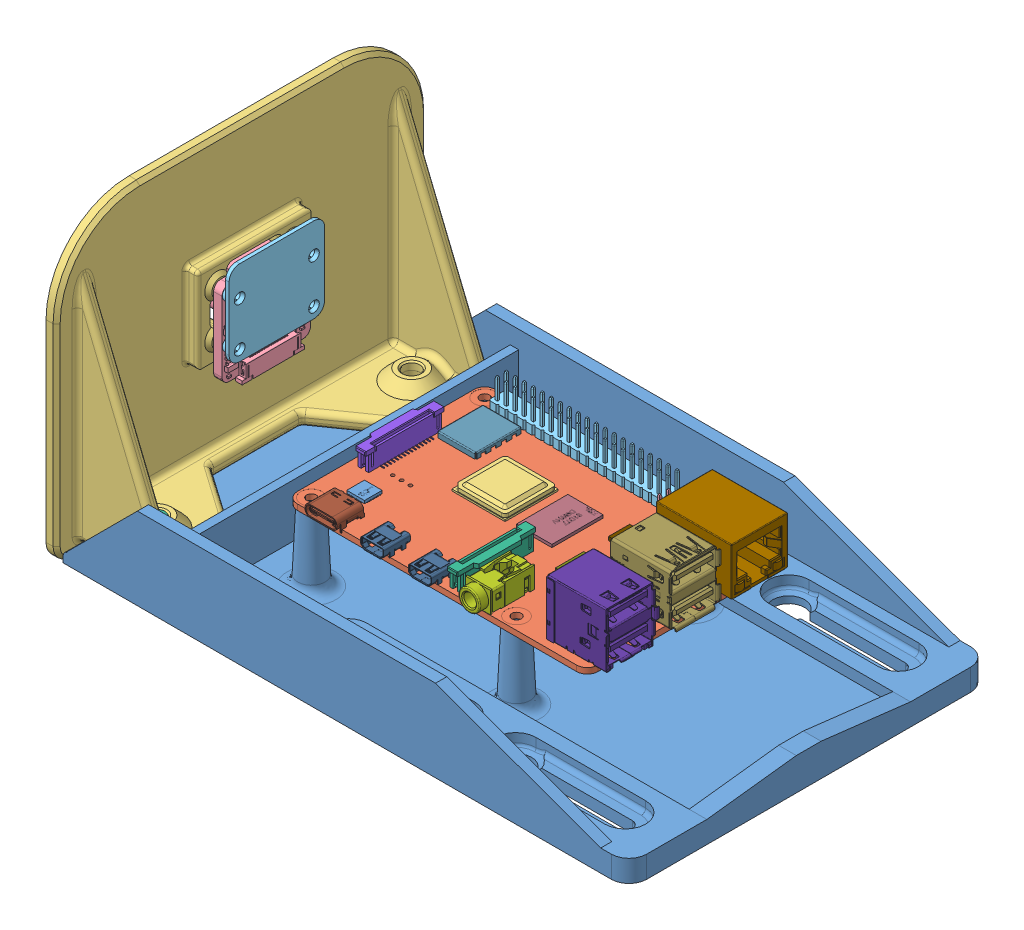
SolidWorks assembly single_pi_assy, configuration Default. Lengths in mm.
Overall size (180.67 83.04 104.77).
26 component instances, 24 part files, 17 mates.
Components (placement in the parent):
- mount_plate_single-1: mount_plate_single [Default] at (-8.7639 97.1511 149.6771) size (160 23.18 101.6)
- Raspberry Pi 4 Model B-1: Raspberry Pi 4 Model B [Default] at (74.1361 121.1161 149.6771) size (88.99 19.9 58.4)
  - PCB, RPi4ModelB-1: PCB, RPi4ModelB [Default] at origin size (85 1.6 56)
  - Broadcom BCM2711B0 CPU, RPi4ModelB-1: Broadcom BCM2711B0 CPU, RPi4ModelB [Default] at (-13.25 0.8 -4.5) size (15 2.3 15)
  - 2.54 mm DUPONT MALE PIN HEADER, POE, 2X2, RPi4ModelB-1: 2.54 mm DUPONT MALE PIN HEADER, POE, 2X2, RPi4ModelB [Default] at (19 0.8 -18.5) size (5.08 11.3 5.08)
  - 2.54 mm DUPONT MALE PIN HEADER, IO, 2X20, RPi4ModelB-1: 2.54 mm DUPONT MALE PIN HEADER, IO, 2X20, RPi4ModelB [Default] at (-10 0.8 -24.5) size (50.8 11.3 5.08)
  - Camera Connector, RPi4ModelB-1: Camera Connector, RPi4ModelB [Default] at (4 0.8 16.5) x (0 0 -1) z (1 0 0) size (22.4 5.68 5.07)
  - Microphone Plug, RPi4ModelB-1: Microphone Plug, RPi4ModelB [Default] at (11.5 0.8 21.65) size (7.23 7.55 15)
  - Display Connector, RPi4ModelB-1: Display Connector, RPi4ModelB [Default] at (-38.5 0.8 0) x (0 0 1) z (-1 0 0) size (22.4 5.68 5.07)
  - Gigabit Ethernet Port, RPi4ModelB-1: Gigabit Ethernet Port, RPi4ModelB [Default] at (45.5 7.55 -17.75) x (0 0 -1) z (1 0 0) size (16.2 17.24 21.64)
  - Female Micro HDMI Connector, RPi4ModelB-2: Female Micro HDMI Connector, RPi4ModelB [Default] at (-3 0.8 27.3875) size (6.5 3.51 7.5)
  - Female Micro HDMI Connector, RPi4ModelB-3: Female Micro HDMI Connector, RPi4ModelB [Default] at (-16.5 0.8 27.3875) size (6.5 3.51 7.5)
  - Female USB Type C Connector, RPi4ModelB-1: Female USB Type C Connector, RPi4ModelB [Default] at (-31.3 0.8 26.5419) size (8.94 3.96 7.9)
  - 2X USB3.0 PORTS, RPi4ModelB-2: 2X USB3.0 PORTS, RPi4ModelB [Default] at (37.07 0.8 1) size (17.47 19.41 15.68)
  - 91D77 D9WHV 778K, 4 GB LPDDR4 SDRAM, RPi4ModelB-1: 91D77 D9WHV 778K, 4 GB LPDDR4 SDRAM, RPi4ModelB [Default] at (2.25 0.8 -4.5) size (10 0.8 14.5)
  - Cypress CYW43455 Wireless Module Cover, RPi4ModelB-1: Cypress CYW43455 Wireless Module Cover, RPi4ModelB [Default] at (-30.5 0.8 -14.5) size (11 1.6 13)
  - SD Card Slot, RPi4ModelB-1: SD Card Slot, RPi4ModelB [Default] at (-35.3 -0.8 0) x (0 0 -1) z (-1 0 0) size (11.95 1.45 11.4)
  - VIA VL805 PCIe USB 3.0 controller, RPi4ModelB-1: VIA VL805 PCIe USB 3.0 controller, RPi4ModelB [Default] at (17.5 0.8 4) size (8.8 0.8 8.8)
  - 2X USB2.0 PORTS, RPi4ModelB-1: 2X USB2.0 PORTS, RPi4ModelB [Default] at (37.065 0.65 19) size (17.87 19.16 15.33)
  - Broadcom BCM54213PE Gigabit Ethernet Transceiver, RPi4ModelB-1: Broadcom BCM54213PE Gigabit Ethernet Transceiver, RPi4ModelB [Default] at (16.5 0.8 -10) size (6.8 1 6.8)
  - MxL7704 Universal PMIC, RPi4ModelB-1: MxL7704 Universal PMIC, RPi4ModelB [Default] at (-32.5 0.8 16) size (5.4 0.8 5.4)
- 94180A323_Tapered Heat-Set Inserts for Plastic-1: 94180A323_Tapered Heat-Set Inserts for Plastic [94180A323] at (93.1361 120.3261 125.1771) size (4.37 5.92 4.37)
- camera_mount_single_portrait-1: camera_mount_single_portrait [Default] at (-12.0139 133.3261 149.6771) x (0 0 -1) z (1 0 0) size (104.77 83.04 28)
- UC-698(B0262)-1: UC-698(B0262) [Default] at (-4.5139 141.5961 149.6771) x (0 0 1) z (-1 0 0) size (25 24.6 29.31)
- camera_cap_fat_clearance-1: camera_cap_fat_clearance [Default] at (-0.1316 143.0761 149.6771) x (0 0 -1) z (1 0 0) size (27 24 3)
- 94180A333_Tapered Heat-Set Inserts for Plastic(1)-1: 94180A333_Tapered Heat-Set Inserts for Plastic(1) [94180A333] at (2.9861 104.0011 185.6771) x (0.994946 0 -0.100412) z (0 -1 0) size (5.56 5.56 6.57)
Mates (geometry in assembly coordinates):
- Width1: width anti-aligned: plane of mount_plate_single-1 through (-8.7639 97.1511 197.3021) normal (0 0 -1); plane of Raspberry Pi 4 Model B-1/PCB, RPi4ModelB-1 through (-8.7639 97.1511 102.0521) normal (0 0 1); plane of mount_plate_single-1 through (31.6361 121.9161 177.6771) normal (0 0 1); plane of Raspberry Pi 4 Model B-1/PCB, RPi4ModelB-1 through (31.6361 121.9161 121.6771) normal (0 0 -1)
- Distance1: distance = 10 mm anti-aligned: plane of Raspberry Pi 4 Model B-1/PCB, RPi4ModelB-1 through (31.6361 121.9161 121.6771) normal (-1 0 0); plane of mount_plate_single-1 through (21.6361 115.3261 197.3021) normal (1 0 0)
- Concentric1: concentric aligned: circle of mount_plate_single-1; circle of 94180A323_Tapered Heat-Set Inserts for Plastic-1
- Coincident1: coincident aligned: plane of mount_plate_single-1 through (93.1361 120.3261 125.1771) normal (0 1 0); plane of 94180A323_Tapered Heat-Set Inserts for Plastic-1 through (93.1361 120.3261 125.1771) normal (0 1 0)
- Coincident2: coincident anti-aligned: plane of mount_plate_single-1 through (93.1361 120.3261 125.1771) normal (0 1 0); plane of Raspberry Pi 4 Model B-1/PCB, RPi4ModelB-1 through (93.1361 120.3261 125.1771) normal (0 -1 0)
- Concentric3: concentric aligned: circle of mount_plate_single-1; circle of test_mount-1
- Coincident3: coincident anti-aligned: plane of mount_plate_single-1 through (-8.7639 100.3261 149.6771) normal (0 1 0); plane of camera_mount_single_portrait-1 through (0.9891 100.3261 97.8574) normal (0 -1 0)
- Concentric4: concentric anti-aligned: circle of test_mount-1; circle of UC-698(B0262)-1
- Concentric5: concentric anti-aligned: circle of camera_mount_single_portrait-1; circle of UC-698(B0262)-1
- Coincident4: coincident anti-aligned: plane of camera_mount_single_portrait-1 through (-19.5574 146.5761 127.7588) normal (0.747569 0 0.664184); plane of UC-698(B0262)-1 through (-18.229 126.7141 126.2636) normal (-0.747569 0 -0.664184)
- Concentric6: concentric aligned: circle of camera_mount_single_portrait-1; circle of camera_cap_fat_clearance-1
- Concentric8: concentric anti-aligned: circle of camera_mount_single_portrait-1; circle of camera_cap_fat_clearance-1
- Coincident5: coincident anti-aligned: plane of UC-698(B0262)-1 through (-16.4481 126.7141 127.8459) normal (0.747569 0 0.664184); plane of camera_cap_fat_clearance-1 through (-17.7765 146.5761 129.3411) normal (-0.747569 0 -0.664184)
- Concentric11: concentric aligned: circle of camera_mount_single_portrait-1; circle of 94180A333_Tapered Heat-Set Inserts for Plastic(1)-1
- Coincident7: coincident aligned: plane of camera_mount_single_portrait-1 through (-44.8352 100.8261 167.5021) normal (0 -1 0); plane of 94180A333_Tapered Heat-Set Inserts for Plastic(1)-1 through (-44.6846 100.8261 168.9945) normal (0 -1 0)
- Concentric12: concentric anti-aligned: circle of mount_plate_single-1; circle of camera_mount_single_portrait-1
- Concentric13: concentric anti-aligned: circle of mount_plate_single-1; circle of camera_mount_single_portrait-1
